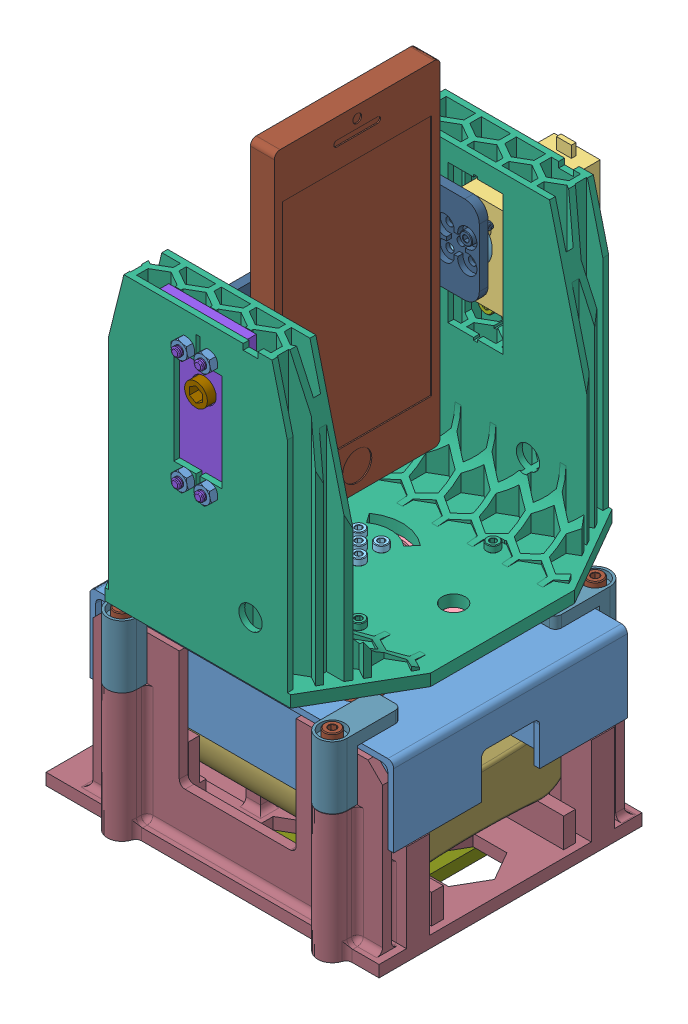
SolidWorks assembly ASSY_IRT_PT_CAM, configuration FIXED. Lengths in mm.
Overall size (144.78 280.29 170.14).
101 component instances, 31 part files, 133 mates.
Components (placement in the parent):
- PAN_BASE_MAIN-1: PAN_BASE_MAIN [Default] at origin
- SPACER_0.75 DIA_8MM-1: SPACER_0.75 DIA_8MM [Default] at (-29.21 34.29 -29.21)
- SPACER_0.75 DIA_8MM-2: SPACER_0.75 DIA_8MM [Default] at (-29.21 34.29 29.21)
- SPACER_0.75 DIA_8MM-3: SPACER_0.75 DIA_8MM [Default] at (29.21 34.29 29.21)
- SPACER_0.75 DIA_8MM-4: SPACER_0.75 DIA_8MM [Default] at (29.21 34.29 -29.21)
- 20KG_6.8V_8V_DIGITAL_SERVO_DSSERVO-1: 20KG_6.8V_8V_DIGITAL_SERVO_DSSERVO [Default] at (-9.464 0.875 0)
- TURNTABLE_ROTATING_ASSY-1: TURNTABLE_ROTATING_ASSY [Default] at (0 42.29 0) size (71.12 8.89 71.12)
  - TURNTABLE_ROTATING_2.8 X 2.8-1: TURNTABLE_ROTATING_2.8 X 2.8 [Default] at origin size (71.12 0.95 71.12)
  - TURNTABLE_ROTATING_2.8 X 2.8-2: TURNTABLE_ROTATING_2.8 X 2.8 [Default] at (0 7.9375 0) x (-1 0 0) z (0 0 -1) size (71.12 0.95 71.12)
- HORN_SERVO-1: HORN_SERVO [Default] at (0 44.3652 0) x (0.996669 0 -0.081556) z (0.081556 0 0.996669)
- TILT_MAIN_BRACKET-1: TILT_MAIN_BRACKET [Default] at (0 51.18 0) x (0 0 1) z (-1 0 0)
- 20KG_6.8V_8V_DIGITAL_SERVO_DSSERVO-2: 20KG_6.8V_8V_DIGITAL_SERVO_DSSERVO [Default] at (0 140.08 -95.01) x (0 1 0) z (1 0 0)
- INNER_COVER_20KG_6.8V_8V_DIGITAL_SERVO_DSSERVO-1: INNER_COVER_20KG_6.8V_8V_DIGITAL_SERVO_DSSERVO [Default] at (0 140.08 60.96)
- COVER_20KG_6.8V_8V_DIGITAL_SERVO_DSSERVO-1: COVER_20KG_6.8V_8V_DIGITAL_SERVO_DSSERVO [Default] at (0 140.08 67.31) x (-1 0 0) z (0 0 -1)
- MOCKUP_LONG_HORN_SERVO-1: MOCKUP_LONG_HORN_SERVO [Default] at (0 149.544 70.705) x (0 1 0) z (-1 0 0)
- HORN_SERVO-2: HORN_SERVO [Default] at (0 149.544 -51.5198) x (0.707107 -0.707107 0) z (-0.707107 -0.707107 0)
- TILT_LONG_BRACKET-1: TILT_LONG_BRACKET [Default] at (-15.24 149.544 -0.415) x (0 0 1) z (0 1 0)
- GALAXY_PHONE-1: GALAXY_PHONE [Default] at (-6.223 149.544 -0.415) x (0 0 -1) z (1 0 0)
- BATTERY_POWER_MASTER_GPCT669-1: BATTERY_POWER_MASTER_GPCT669 [Default] at (0 -13.0494 0) x (0 0 -1) z (1 0 0)
- BASE_BATTERY_ESP32-1: BASE_BATTERY_ESP32 [Default] at (0 -43.8787 0) x (-1 0 0) z (0 0 -1)
- PUSH_DOWN-1: PUSH_DOWN [Default] at (45.72 12.192 52.578) x (-1 0 0) z (0 0 -1)
- PUSH_DOWN-2: PUSH_DOWN [Default] at (-45.72 12.0013 52.578) x (-1 0 0) z (0 0 -1)
- PUSH_DOWN-3: PUSH_DOWN [Default] at (-45.72 12.192 -52.578)
- PUSH_DOWN-4: PUSH_DOWN [Default] at (45.72 12.192 -52.578)
- ESP32-1: ESP32 [Default] at (-50.2285 -31.1787 0)
- TRIPOD_ADAPTER-1: TRIPOD_ADAPTER [Default] at (0 -48.9587 0)
- INSERT_PUSH_DOWN-1: INSERT_PUSH_DOWN [Default] at (45.72 10.5213 -57.15)
- INSERT_PUSH_DOWN-2: INSERT_PUSH_DOWN [Default] at (45.72 10.5213 57.15)
- INSERT_PUSH_DOWN-3: INSERT_PUSH_DOWN [Default] at (-45.72 10.5213 -57.15)
- INSERT_PUSH_DOWN-4: INSERT_PUSH_DOWN [Default] at (-45.72 10.5213 57.15)
- INSERT_CENTER_PUSH_DOWN-1: INSERT_CENTER_PUSH_DOWN [Default] at (0 -33.7187 0)
- M4_Steel Hex Nut_90592A090-1: M4_Steel Hex Nut_90592A090 [90592A090] at (15.286 26.975 5)
- M4_Steel Hex Nut_90592A090-4: M4_Steel Hex Nut_90592A090 [90592A090] at (15.286 26.975 -5)
- M4_Steel Hex Nut_90592A090-3: M4_Steel Hex Nut_90592A090 [90592A090] at (-34.214 26.975 -5)
- M4_Steel Hex Nut_90592A090-2: M4_Steel Hex Nut_90592A090 [90592A090] at (-34.214 26.975 5)
- M3_Steel Hex Nut_90592A085-1: M3_Steel Hex Nut_90592A085 [90592A085] at (-29.21 30.55 -29.21) x (0.956593 0 0.291427) z (-0.291427 0 0.956593)
- M3_General Purpose 18-8 Stainless Steel Washer_98689A112-1: M3_General Purpose 18-8 Stainless Steel Washer_98689A112 [98689A112] at (-29.21 43.5425 -29.21) x (1 0 0) z (0 1 0)
- M3 X 16MM_Button Head Hex Drive Screw_92095A184-1: M3 X 16MM_Button Head Hex Drive Screw_92095A184 [92095A184] at (-29.21 45.4925 -29.21) x (1 0 0) z (0 1 0)
- M3_General Purpose 18-8 Stainless Steel Washer_98689A112-2: M3_General Purpose 18-8 Stainless Steel Washer_98689A112 [98689A112] at (29.21 49.9275 -29.21) x (0.994029 0 -0.109119) z (0 -1 0)
- M3_Steel Hex Nut_90592A085-5: M3_Steel Hex Nut_90592A085 [90592A085] at (29.21 48.4275 -29.21) x (0.873242 0 0.487286) z (-0.487286 0 0.873242)
- M3_Steel Hex Nut_90592A085-9: M3_Steel Hex Nut_90592A085 [90592A085] at (0 149.544 49.6935) x (0.5 0.866025 0) z (-0.866025 0.5 0)
- M3 X 12MM_18-8 Stainless Steel Socket Head Screw_91292A114-1: M3 X 12MM_18-8 Stainless Steel Socket Head Screw_91292A114 [91292A114] at (4.9391 44.26 4.9391) x (1 0 0) z (0 -1 0)
- M3 X 10MM_18-8 Stainless Steel Socket Head Screw_91292A113-1: M3 X 10MM_18-8 Stainless Steel Socket Head Screw_91292A113 [91292A113] at (-29.21 46.26 -29.21) x (-0.837169 0 -0.546944) z (0 -1 0)
- M4 X 10MM_18-8 Stainless Steel Socket Head Screw_91292A116-1: M4 X 10MM_18-8 Stainless Steel Socket Head Screw_91292A116 [91292A116] at (5 164.83 -74.135) x (-1 0 0) z (0 0 -1)
- M4_Steel Hex Nut_90592A090-5: M4_Steel Hex Nut_90592A090 [90592A090] at (5 164.83 -71.45) x (-0.976148 -0.217105 0) z (-0.217105 0.976148 0)
- M4_Steel Hex Nut_90592A090-9: M4_Steel Hex Nut_90592A090 [90592A090] at (5 164.83 71.45) x (-0.976148 -0.217105 0) z (-0.217105 0.976148 0)
- M4 X 14MM_18-8 Stainless Steel Socket Head Screw_91292A038-1: M4 X 14MM_18-8 Stainless Steel Socket Head Screw_91292A038 [91292A038] at (5 164.83 74.96) x (0.908511 -0.417861 0) z (0 0 1)
- M4 X 12MM_Zinc-Plated Alloy Steel Socket Head Screw_90128A214-1: M4 X 12MM_Zinc-Plated Alloy Steel Socket Head Screw_90128A214 [90128A214] at (15.286 22.29 5) x (1 0 0) z (0 -1 0)
- M3 X 8MM_18-8 Stainless Steel Socket Head Screw_91292A112-6: M3 X 8MM_18-8 Stainless Steel Socket Head Screw_91292A112 [91292A112] at (0 149.544 51.795)
- M3 X 8MM_18-8 Stainless Steel Socket Head Screw_91292A112-1: M3 X 8MM_18-8 Stainless Steel Socket Head Screw_91292A112 [91292A112] at (4.9391 154.4831 -52.625) x (-0.943465 -0.331474 0) z (0 0 -1)
- M4 X 12MM_Zinc-Plated Alloy Steel Socket Head Screw_90128A214-4: M4 X 12MM_Zinc-Plated Alloy Steel Socket Head Screw_90128A214 [90128A214] at (15.286 22.29 -5) x (1 0 0) z (0 -1 0)
- M4 X 12MM_Zinc-Plated Alloy Steel Socket Head Screw_90128A214-3: M4 X 12MM_Zinc-Plated Alloy Steel Socket Head Screw_90128A214 [90128A214] at (-34.214 22.29 -5) x (1 0 0) z (0 -1 0)
- M4 X 12MM_Zinc-Plated Alloy Steel Socket Head Screw_90128A214-2: M4 X 12MM_Zinc-Plated Alloy Steel Socket Head Screw_90128A214 [90128A214] at (-34.214 22.29 5) x (1 0 0) z (0 -1 0)
- M4 X 40MM_18-8 Stainless Steel Socket Head Screw_91292A132-1: M4 X 40MM_18-8 Stainless Steel Socket Head Screw_91292A132 [91292A132] at (-45.72 18.37 -57.15) x (1 0 0) z (0 1 0)
- M4 X 40MM_18-8 Stainless Steel Socket Head Screw_91292A132-2: M4 X 40MM_18-8 Stainless Steel Socket Head Screw_91292A132 [91292A132] at (-45.72 18.1793 57.15) x (1 0 0) z (0 1 0)
- M4 X 40MM_18-8 Stainless Steel Socket Head Screw_91292A132-3: M4 X 40MM_18-8 Stainless Steel Socket Head Screw_91292A132 [91292A132] at (45.72 18.37 57.15) x (0.445727 0 0.895169) z (0 1 0)
- M4 X 40MM_18-8 Stainless Steel Socket Head Screw_91292A132-4: M4 X 40MM_18-8 Stainless Steel Socket Head Screw_91292A132 [91292A132] at (45.72 18.37 -57.15) x (0.972297 0 0.23375) z (0 1 0)
- M4_Steel Hex Nut_90592A090-13: M4_Steel Hex Nut_90592A090 [90592A090] at (45.72 8.5213 -57.15) x (0.866025 0 -0.5) z (0.5 0 0.866025)
- M4_Steel Hex Nut_90592A090-14: M4_Steel Hex Nut_90592A090 [90592A090] at (-45.72 8.5213 -57.15) x (0 0 -1) z (1 0 0)
- M4_Steel Hex Nut_90592A090-15: M4_Steel Hex Nut_90592A090 [90592A090] at (45.72 8.5213 57.15) x (0.866025 0 -0.5) z (0.5 0 0.866025)
- M4_Steel Hex Nut_90592A090-16: M4_Steel Hex Nut_90592A090 [90592A090] at (-45.72 8.5213 57.15) x (0.866025 0 -0.5) z (0.5 0 0.866025)
- 1 4 -20_18-8 Stainless Steel Hex Nut_92673A113-1: 1 4 -20_18-8 Stainless Steel Hex Nut_92673A113 [92673A113] at (0 -36.0206 0) x (0.866025 0 0.5) z (0 1 0)
- 1 4 -20 5 AND 8_Zinc-Aluminum-Coated Alloy Steel Socket Head Screw_91274A160-1: 1 4 -20 5 AND 8_Zinc-Aluminum-Coated Alloy Steel Socket Head Screw_91274A160 [91274A160] at (0 -31.3057 0) x (1 0 0) z (0 1 0)
- M3 X 16MM_Button Head Hex Drive Screw_92095A184-2: M3 X 16MM_Button Head Hex Drive Screw_92095A184 [92095A184] at (-29.21 45.4925 29.21) x (1 0 0) z (0 1 0)
- M3 X 16MM_Button Head Hex Drive Screw_92095A184-3: M3 X 16MM_Button Head Hex Drive Screw_92095A184 [92095A184] at (29.21 45.4925 29.21) x (1 0 0) z (0 1 0)
- M3 X 16MM_Button Head Hex Drive Screw_92095A184-4: M3 X 16MM_Button Head Hex Drive Screw_92095A184 [92095A184] at (29.21 45.4925 -29.21) x (1 0 0) z (0 1 0)
- M3_General Purpose 18-8 Stainless Steel Washer_98689A112-3: M3_General Purpose 18-8 Stainless Steel Washer_98689A112 [98689A112] at (29.21 49.9275 29.21) x (0.994029 0 -0.109119) z (0 -1 0)
- M3_General Purpose 18-8 Stainless Steel Washer_98689A112-4: M3_General Purpose 18-8 Stainless Steel Washer_98689A112 [98689A112] at (-29.21 49.9275 29.21) x (0.994029 0 -0.109119) z (0 -1 0)
- M3_General Purpose 18-8 Stainless Steel Washer_98689A112-5: M3_General Purpose 18-8 Stainless Steel Washer_98689A112 [98689A112] at (-29.21 49.9275 -29.21) x (0.994029 0 -0.109119) z (0 -1 0)
- M3_General Purpose 18-8 Stainless Steel Washer_98689A112-6: M3_General Purpose 18-8 Stainless Steel Washer_98689A112 [98689A112] at (-29.21 43.5425 29.21) x (1 0 0) z (0 1 0)
- M3_General Purpose 18-8 Stainless Steel Washer_98689A112-7: M3_General Purpose 18-8 Stainless Steel Washer_98689A112 [98689A112] at (29.21 43.5425 29.21) x (1 0 0) z (0 1 0)
- M3_General Purpose 18-8 Stainless Steel Washer_98689A112-8: M3_General Purpose 18-8 Stainless Steel Washer_98689A112 [98689A112] at (29.21 43.5425 -29.21) x (1 0 0) z (0 1 0)
- M3_Steel Hex Nut_90592A085-2: M3_Steel Hex Nut_90592A085 [90592A085] at (-29.21 30.55 29.21) x (0.956593 0 0.291427) z (-0.291427 0 0.956593)
- M3_Steel Hex Nut_90592A085-3: M3_Steel Hex Nut_90592A085 [90592A085] at (29.21 30.55 29.21) x (0.956593 0 0.291427) z (-0.291427 0 0.956593)
- M3_Steel Hex Nut_90592A085-4: M3_Steel Hex Nut_90592A085 [90592A085] at (29.21 30.55 -29.21) x (0.956593 0 0.291427) z (-0.291427 0 0.956593)
- M3_Steel Hex Nut_90592A085-6: M3_Steel Hex Nut_90592A085 [90592A085] at (29.21 48.4275 29.21) x (0.873242 0 0.487286) z (-0.487286 0 0.873242)
- M3_Steel Hex Nut_90592A085-7: M3_Steel Hex Nut_90592A085 [90592A085] at (-29.21 48.4275 29.21) x (0.873242 0 0.487286) z (-0.487286 0 0.873242)
- M3_Steel Hex Nut_90592A085-8: M3_Steel Hex Nut_90592A085 [90592A085] at (-29.21 48.4275 -29.21) x (0.873242 0 0.487286) z (-0.487286 0 0.873242)
- M3 X 10MM_18-8 Stainless Steel Socket Head Screw_91292A113-2: M3 X 10MM_18-8 Stainless Steel Socket Head Screw_91292A113 [91292A113] at (29.21 46.26 -29.21) x (-0.837169 0 -0.546944) z (0 -1 0)
- M3 X 10MM_18-8 Stainless Steel Socket Head Screw_91292A113-3: M3 X 10MM_18-8 Stainless Steel Socket Head Screw_91292A113 [91292A113] at (29.21 46.26 29.21) x (-0.837169 0 -0.546944) z (0 -1 0)
- M3 X 10MM_18-8 Stainless Steel Socket Head Screw_91292A113-4: M3 X 10MM_18-8 Stainless Steel Socket Head Screw_91292A113 [91292A113] at (-29.21 46.26 29.21) x (-0.837169 0 -0.546944) z (0 -1 0)
- M3 X 12MM_18-8 Stainless Steel Socket Head Screw_91292A114-2: M3 X 12MM_18-8 Stainless Steel Socket Head Screw_91292A114 [91292A114] at (0 44.26 0) x (1 0 0) z (0 -1 0)
- M3 X 12MM_18-8 Stainless Steel Socket Head Screw_91292A114-3: M3 X 12MM_18-8 Stainless Steel Socket Head Screw_91292A114 [91292A114] at (-4.9391 44.26 4.9391) x (1 0 0) z (0 -1 0)
- M3 X 12MM_18-8 Stainless Steel Socket Head Screw_91292A114-4: M3 X 12MM_18-8 Stainless Steel Socket Head Screw_91292A114 [91292A114] at (-4.9391 44.26 -4.9391) x (1 0 0) z (0 -1 0)
- M3 X 12MM_18-8 Stainless Steel Socket Head Screw_91292A114-5: M3 X 12MM_18-8 Stainless Steel Socket Head Screw_91292A114 [91292A114] at (4.9391 44.26 -4.9391) x (1 0 0) z (0 -1 0)
- M4_Steel Hex Nut_90592A090-6: M4_Steel Hex Nut_90592A090 [90592A090] at (5 115.33 -71.45) x (-0.976148 -0.217105 0) z (-0.217105 0.976148 0)
- M4_Steel Hex Nut_90592A090-7: M4_Steel Hex Nut_90592A090 [90592A090] at (-5 115.33 -71.45) x (-0.976148 -0.217105 0) z (-0.217105 0.976148 0)
- M4_Steel Hex Nut_90592A090-8: M4_Steel Hex Nut_90592A090 [90592A090] at (-5 164.83 -71.45) x (-0.976148 -0.217105 0) z (-0.217105 0.976148 0)
- M4 X 10MM_18-8 Stainless Steel Socket Head Screw_91292A116-2: M4 X 10MM_18-8 Stainless Steel Socket Head Screw_91292A116 [91292A116] at (5 115.33 -74.135) x (-1 0 0) z (0 0 -1)
- M4 X 10MM_18-8 Stainless Steel Socket Head Screw_91292A116-3: M4 X 10MM_18-8 Stainless Steel Socket Head Screw_91292A116 [91292A116] at (-5 115.33 -74.135) x (-1 0 0) z (0 0 -1)
- M4 X 10MM_18-8 Stainless Steel Socket Head Screw_91292A116-4: M4 X 10MM_18-8 Stainless Steel Socket Head Screw_91292A116 [91292A116] at (-5 164.83 -74.135) x (-1 0 0) z (0 0 -1)
- M4 X 14MM_18-8 Stainless Steel Socket Head Screw_91292A038-2: M4 X 14MM_18-8 Stainless Steel Socket Head Screw_91292A038 [91292A038] at (-5 115.33 74.96) x (0.908511 -0.417861 0) z (0 0 1)
- M4 X 14MM_18-8 Stainless Steel Socket Head Screw_91292A038-3: M4 X 14MM_18-8 Stainless Steel Socket Head Screw_91292A038 [91292A038] at (5 115.33 74.96) x (0.908511 -0.417861 0) z (0 0 1)
- M4 X 14MM_18-8 Stainless Steel Socket Head Screw_91292A038-4: M4 X 14MM_18-8 Stainless Steel Socket Head Screw_91292A038 [91292A038] at (-5 164.83 74.96) x (0.908511 -0.417861 0) z (0 0 1)
- M4_Steel Hex Nut_90592A090-10: M4_Steel Hex Nut_90592A090 [90592A090] at (-5 115.33 71.45) x (-0.976148 -0.217105 0) z (-0.217105 0.976148 0)
- M4_Steel Hex Nut_90592A090-11: M4_Steel Hex Nut_90592A090 [90592A090] at (5 115.33 71.45) x (-0.976148 -0.217105 0) z (-0.217105 0.976148 0)
- M4_Steel Hex Nut_90592A090-12: M4_Steel Hex Nut_90592A090 [90592A090] at (-5 164.83 71.45) x (-0.976148 -0.217105 0) z (-0.217105 0.976148 0)
- M3 X 8MM_18-8 Stainless Steel Socket Head Screw_91292A112-2: M3 X 8MM_18-8 Stainless Steel Socket Head Screw_91292A112 [91292A112] at (-4.9391 144.6049 -52.625) x (-0.943465 -0.331474 0) z (0 0 -1) (suppressed, hidden)
- M3 X 8MM_18-8 Stainless Steel Socket Head Screw_91292A112-3: M3 X 8MM_18-8 Stainless Steel Socket Head Screw_91292A112 [91292A112] at (-4.9391 154.4831 -52.625) x (-0.943465 -0.331474 0) z (0 0 -1) (suppressed, hidden)
- M3 X 8MM_18-8 Stainless Steel Socket Head Screw_91292A112-4: M3 X 8MM_18-8 Stainless Steel Socket Head Screw_91292A112 [91292A112] at (0 149.544 -52.625) x (-0.943465 -0.331474 0) z (0 0 -1) (suppressed, hidden)
- M3 X 8MM_18-8 Stainless Steel Socket Head Screw_91292A112-5: M3 X 8MM_18-8 Stainless Steel Socket Head Screw_91292A112 [91292A112] at (4.9391 144.6049 -52.625) x (-0.943465 -0.331474 0) z (0 0 -1) (suppressed, hidden)
Mates (geometry in assembly coordinates):
- Coincident1: coincident aligned: plane of BASE_1.3-1 through (0 0 0) normal (1 0 0)
- Coincident2: coincident aligned: plane of BASE_1.3-1 through (0 0 0) normal (0 1 0)
- Coincident3: coincident aligned: plane of BASE_1.3-1 through (0 0 0) normal (0 0 1)
- Concentric1: concentric anti-aligned: cylinder of SPACER_0.75 DIA_8MM-1 through (-29.21 42.29 -29.21) axis (0 -1 0) radius 2; cylinder of BASE_1.3-1 through (-29.21 34.29 -29.21) axis (0 1 0) radius 1.8
- Coincident4: coincident anti-aligned: plane of BASE_1.3-1 through (0 34.29 50.8) normal (0 1 0); plane of SPACER_0.75 DIA_8MM-1 through (-29.21 34.29 -29.21) normal (0 -1 0)
- Parallel1: parallel aligned: plane of SPACER_0.75 DIA_8MM-1 through (-29.21 34.29 -29.21) normal (1 0 0)
- Coincident6: coincident: line of 20KG_6.8V_8V_DIGITAL_SERVO_DSSERVO-1 through (0 46.355 0) axis (0 -1 0)
- Coincident7: coincident anti-aligned: plane of BASE_1.3-1 through (0 31.75 50.8) normal (0 -1 0); plane of 20KG_6.8V_8V_DIGITAL_SERVO_DSSERVO-1 through (-9.464 31.75 0) normal (0 1 0)
- Coincident8: coincident aligned: plane of 20KG_6.8V_8V_DIGITAL_SERVO_DSSERVO-1 through (-9.464 0.875 0) normal (0 0 1)
- Coincident9: coincident anti-aligned: line of BASE_1.3-1 through (15.286 31.75 5) axis (0 1 0); line of M4 X 12MM_Zinc-Plated Alloy Steel Socket Head Screw_90128A214-1 through (15.286 34.29 5) axis (0 -1 0)
- Coincident10: coincident anti-aligned: plane of BASE_1.3-1 through (0 34.29 50.8) normal (0 1 0); plane of M4 X 12MM_Zinc-Plated Alloy Steel Socket Head Screw_90128A214-1 through (15.286 34.29 5) normal (0 -1 0)
- Coincident11: coincident anti-aligned: line of BASE_1.3-1 through (15.286 31.75 5) axis (0 1 0); line of M4 X 3.2MM_Steel Hex Nut_90592A090-1 through (15.286 28.575 5) axis (0 -1 0)
- Coincident12: coincident anti-aligned: plane of 20KG_6.8V_8V_DIGITAL_SERVO_DSSERVO-1 through (-9.464 28.575 0) normal (0 -1 0); plane of M4 X 3.2MM_Steel Hex Nut_90592A090-1 through (11.786 28.575 2.9793) normal (0 1 0)
- Coincident13: coincident anti-aligned: plane of SPACER_0.75 DIA_8MM-3 through (29.21 42.29 29.21) normal (0 1 0); plane of TURNTABLE_ROTATING_ASSY-1/TURNTABLE_ROTATING_2.8 X 2.8-1 through (0 42.29 0) normal (0 -1 0)
- Coincident14: coincident aligned: plane of TURNTABLE_ROTATING_ASSY-1 through (0 42.29 0) normal (1 0 0)
- Coincident15: coincident aligned: plane of TURNTABLE_ROTATING_ASSY-1 through (0 42.29 0) normal (0 0 1)
- Coincident16: coincident anti-aligned: plane of M3 X 16MM_Button Head Hex Drive Screw_92095A184-1 through (-26.36 43.8425 -29.21) normal (0 -1 0); plane of M3_General Purpose 18-8 Stainless Steel Washer_98689A112-1 through (-29.21 43.8425 -29.21) normal (0 1 0)
- Coincident17: coincident anti-aligned: line of BASE_1.3-1 through (-29.21 31.75 -29.21) axis (0 1 0); line of M3_General Purpose 18-8 Stainless Steel Washer_98689A112-1 through (-29.21 43.8425 -29.21) axis (0 -1 0)
- Coincident18: coincident anti-aligned: plane of TURNTABLE_ROTATING_ASSY-1/TURNTABLE_ROTATING_2.8 X 2.8-1 through (0 43.2425 0) normal (0 1 0); plane of M3_General Purpose 18-8 Stainless Steel Washer_98689A112-1 through (-29.21 43.2425 -29.21) normal (0 -1 0)
- Coincident19: coincident anti-aligned: line of BASE_1.3-1 through (-29.21 31.75 -29.21) axis (0 1 0); line of TURNTABLE_ROTATING_ASSY-1/M3_General Purpose 18-8 Stainless Steel Washer_98689A112-1 through (-29.21 43.8425 -29.21) axis (0 -1 0)
- Concentric2: concentric aligned: cylinder of TURNTABLE_ROTATING_ASSY-1/TURNTABLE_ROTATING_2.8 X 2.8-2 through (29.21 51.18 -29.21) axis (0 1 0) radius 1.7; cylinder of M3_General Purpose 18-8 Stainless Steel Washer_98689A112-2 through (29.21 49.6275 -29.21) axis (0 1 0) radius 1.6
- Coincident20: coincident anti-aligned: plane of TURNTABLE_ROTATING_ASSY-1/TURNTABLE_ROTATING_2.8 X 2.8-2 through (0 50.2275 0) normal (0 -1 0); plane of M3_General Purpose 18-8 Stainless Steel Washer_98689A112-2 through (29.21 50.2275 -29.21) normal (0 1 0)
- Coincident21: coincident anti-aligned: line of BASE_1.3-1 through (-29.21 31.75 -29.21) axis (0 1 0); line of M3_Steel Hex Nut_90592A085-1 through (-29.21 31.75 -29.21) axis (0 -1 0)
- Coincident23: coincident anti-aligned: plane of BASE_1.3-1 through (0 31.75 50.8) normal (0 -1 0); plane of M3_Steel Hex Nut_90592A085-1 through (-31.3779 31.75 -31.5302) normal (0 1 0)
- Concentric3: concentric aligned: cylinder of 20KG_6.8V_8V_DIGITAL_SERVO_DSSERVO-1 through (0 46.355 0) axis (0 -1 0) radius 2.921; cylinder of HORN_SERVO-1 through (0 44.3652 0) axis (0 -1 0) radius 4.7244
- Distance2: distance = 18 mm aligned: plane of HORN_SERVO-1 through (0 49.75 0) normal (0 1 0); plane of 20KG_6.8V_8V_DIGITAL_SERVO_DSSERVO-1 through (-9.464 31.75 0) normal (0 1 0)
- Concentric4: concentric aligned: cylinder of TURNTABLE_ROTATING_ASSY-1/TURNTABLE_ROTATING_2.8 X 2.8-2 through (29.21 51.18 29.21) axis (0 1 0) radius 1.7; cylinder of TILT_MAIN_BRACKET-1 through (29.21 56.26 29.21) axis (0 1 0) radius 1.8
- Concentric5: concentric aligned: cylinder of TURNTABLE_ROTATING_ASSY-1/TURNTABLE_ROTATING_2.8 X 2.8-2 through (-29.21 51.18 -29.21) axis (0 1 0) radius 1.7; cylinder of TILT_MAIN_BRACKET-1 through (-29.21 56.26 -29.21) axis (0 1 0) radius 1.8
- Coincident26: coincident anti-aligned: plane of TURNTABLE_ROTATING_ASSY-1/TURNTABLE_ROTATING_2.8 X 2.8-2 through (0 51.18 0) normal (0 1 0); plane of TILT_MAIN_BRACKET-1 through (0 51.18 0) normal (0 -1 0)
- Coincident27: coincident anti-aligned: line of TURNTABLE_ROTATING_ASSY-1/TURNTABLE_ROTATING_2.8 X 2.8-2 through (29.21 50.2275 -29.21) axis (0 1 0); line of M3_Steel Hex Nut_90592A085-5 through (29.21 49.6275 -29.21) axis (0 -1 0)
- Coincident28: coincident anti-aligned: plane of M3_General Purpose 18-8 Stainless Steel Washer_98689A112-2 through (29.21 49.6275 -29.21) normal (0 -1 0); plane of M3_Steel Hex Nut_90592A085-5 through (27.5823 49.6275 -31.9365) normal (0 1 0)
- Coincident33: coincident aligned: line of TILT_MAIN_BRACKET-1 through (-29.21 58.2611 -29.21) axis (0 -1 0); line of M3 X 10MM_18-8 Stainless Steel Socket Head Screw_91292A113-1 through (-29.21 58.985 -29.21) axis (0 -1 0)
- Coincident34: coincident anti-aligned: plane of TILT_MAIN_BRACKET-1 through (0 56.26 0) normal (0 1 0); plane of M3 X 10MM_18-8 Stainless Steel Socket Head Screw_91292A113-1 through (-29.21 56.26 -29.21) normal (0 -1 0)
- Coincident35: coincident anti-aligned: line of TILT_MAIN_BRACKET-1 through (4.9391 51.18 4.9391) axis (0 1 0); line of M3 X 12MM_18-8 Stainless Steel Socket Head Screw_91292A114-1 through (4.9391 58.985 4.9391) axis (0 -1 0)
- Coincident36: coincident anti-aligned: plane of TILT_MAIN_BRACKET-1 through (0 56.26 0) normal (0 1 0); plane of M3 X 12MM_18-8 Stainless Steel Socket Head Screw_91292A114-1 through (4.9391 56.26 4.9391) normal (0 -1 0)
- Coincident37: coincident anti-aligned: plane of TILT_MAIN_BRACKET-1 through (0 51.18 0) normal (-1 0 0); plane of 20KG_6.8V_8V_DIGITAL_SERVO_DSSERVO-2 through (0 140.08 -95.01) normal (1 0 0)
- Concentric6: concentric aligned: cylinder of TILT_MAIN_BRACKET-1 through (-5 164.83 -67.31) axis (0 0 1) radius 2.4; cylinder of 20KG_6.8V_8V_DIGITAL_SERVO_DSSERVO-2 through (-5 164.83 -95.011) axis (0 0 1) radius 2.5
- Concentric7: concentric aligned: cylinder of TILT_MAIN_BRACKET-1 through (5 115.33 -67.31) axis (0 0 1) radius 2.4; cylinder of 20KG_6.8V_8V_DIGITAL_SERVO_DSSERVO-2 through (5 115.33 -95.011) axis (0 0 1) radius 2.5
- Coincident38: coincident anti-aligned: plane of TILT_MAIN_BRACKET-1 through (-101.6 381.3959 -67.31) normal (0 0 1); plane of 20KG_6.8V_8V_DIGITAL_SERVO_DSSERVO-2 through (0 140.08 -67.31) normal (0 0 -1)
- Coincident39: coincident anti-aligned: line of TILT_MAIN_BRACKET-1 through (5 164.83 -69.85) axis (0 0 1); line of M4 X 10MM_18-8 Stainless Steel Socket Head Screw_91292A116-1 through (5 164.83 -60.485) axis (0 0 -1)
- Coincident40: coincident anti-aligned: plane of 20KG_6.8V_8V_DIGITAL_SERVO_DSSERVO-2 through (0 140.08 -64.135) normal (0 0 1); plane of M4 X 10MM_18-8 Stainless Steel Socket Head Screw_91292A116-1 through (5 164.83 -64.135) normal (0 0 -1)
- Coincident41: coincident anti-aligned: line of TILT_MAIN_BRACKET-1 through (5 164.83 -69.85) axis (0 0 1); line of M4_Steel Hex Nut_90592A090-5 through (5 164.83 -69.85) axis (0 0 -1)
- Coincident42: coincident anti-aligned: plane of TILT_MAIN_BRACKET-1 through (-101.6 381.3959 -69.85) normal (0 0 -1); plane of M4_Steel Hex Nut_90592A090-5 through (8.8552 163.6173 -69.85) normal (0 0 1)
- Concentric8: concentric aligned: cylinder of TILT_MAIN_BRACKET-1 through (-5 164.83 67.31) axis (0 0 -1) radius 2.4; cylinder of COVER_20KG_6.8V_8V_DIGITAL_SERVO_DSSERVO-1 through (-5 164.83 63.5) axis (0 0 -1) radius 2.25
- Concentric9: concentric aligned: cylinder of TILT_MAIN_BRACKET-1 through (5 115.33 67.31) axis (0 0 -1) radius 2.4; cylinder of COVER_20KG_6.8V_8V_DIGITAL_SERVO_DSSERVO-1 through (5 115.33 63.5) axis (0 0 -1) radius 2.25
- Coincident43: coincident anti-aligned: plane of TILT_MAIN_BRACKET-1 through (-101.6 381.3959 67.31) normal (0 0 -1); plane of COVER_20KG_6.8V_8V_DIGITAL_SERVO_DSSERVO-1 through (0 140.08 67.31) normal (0 0 1)
- Concentric10: concentric aligned: cylinder of COVER_20KG_6.8V_8V_DIGITAL_SERVO_DSSERVO-1 through (5 164.83 63.5) axis (0 0 -1) radius 2.25; cylinder of INNER_COVER_20KG_6.8V_8V_DIGITAL_SERVO_DSSERVO-1 through (5 164.83 60.96) axis (0 0 -1) radius 2.25
- Concentric11: concentric aligned: cylinder of TILT_MAIN_BRACKET-1 through (5 115.33 67.31) axis (0 0 -1) radius 2.4; cylinder of INNER_COVER_20KG_6.8V_8V_DIGITAL_SERVO_DSSERVO-1 through (5 115.33 60.96) axis (0 0 -1) radius 2.25
- Coincident44: coincident anti-aligned: plane of COVER_20KG_6.8V_8V_DIGITAL_SERVO_DSSERVO-1 through (0 140.08 63.5) normal (0 0 -1); plane of INNER_COVER_20KG_6.8V_8V_DIGITAL_SERVO_DSSERVO-1 through (0 140.08 63.5) normal (0 0 1)
- Coincident47: coincident anti-aligned: line of INNER_COVER_20KG_6.8V_8V_DIGITAL_SERVO_DSSERVO-1 through (5 164.83 63.5) axis (0 0 -1); line of M4 X 14MM_18-8 Stainless Steel Socket Head Screw_91292A038-1 through (5 164.83 60.96) axis (0 0 1)
- Coincident48: coincident anti-aligned: plane of INNER_COVER_20KG_6.8V_8V_DIGITAL_SERVO_DSSERVO-1 through (0 140.08 60.96) normal (0 0 -1); plane of M4 X 14MM_18-8 Stainless Steel Socket Head Screw_91292A038-1 through (5 164.83 60.96) normal (0 0 1)
- Coincident49: coincident aligned: line of INNER_COVER_20KG_6.8V_8V_DIGITAL_SERVO_DSSERVO-1 through (5 164.83 63.5) axis (0 0 -1); line of M4_Steel Hex Nut_90592A090-9 through (5 164.83 73.05) axis (0 0 -1)
- Coincident50: coincident anti-aligned: plane of TILT_MAIN_BRACKET-1 through (-101.6 381.3959 69.85) normal (0 0 1); plane of M4_Steel Hex Nut_90592A090-9 through (8.8552 163.6173 69.85) normal (0 0 -1)
- Concentric12: concentric anti-aligned: cylinder of COVER_20KG_6.8V_8V_DIGITAL_SERVO_DSSERVO-1 through (0 149.544 67.311) axis (0 0 -1) radius 5.3975; cylinder of MOCKUP_LONG_HORN_SERVO-1 through (0 149.544 70.705) axis (0 0 1) radius 4.953
- Concentric13: concentric aligned: cylinder of 20KG_6.8V_8V_DIGITAL_SERVO_DSSERVO-2 through (0 149.544 -49.53) axis (0 0 -1) radius 2.921; cylinder of HORN_SERVO-2 through (0 149.544 -48.5988) axis (0 0 -1) radius 2.667
- Distance3: distance = 18 mm aligned: plane of HORN_SERVO-2 through (0 149.544 -46.135) normal (0 0 1); plane of 20KG_6.8V_8V_DIGITAL_SERVO_DSSERVO-2 through (0 140.08 -64.135) normal (0 0 1)
- Concentric14: concentric aligned: cylinder of HORN_SERVO-2 through (0 149.544 -46.135) axis (0 0 1) radius 1.6; cylinder of TILT_LONG_BRACKET-1 through (0 149.544 -42.325) axis (0 0 1) radius 1.8
- Coincident53: coincident anti-aligned: plane of HORN_SERVO-2 through (0 149.544 -46.135) normal (0 0 1); plane of TILT_LONG_BRACKET-1 through (-11.43 130.494 -46.135) normal (0 0 -1)
- Concentric15: concentric aligned: cylinder of HORN_SERVO-2 through (4.9391 154.4831 -46.135) axis (0 0 1) radius 1.6; cylinder of TILT_LONG_BRACKET-1 through (4.9391 154.4831 -42.325) axis (0 0 1) radius 1.8
- Coincident54: coincident anti-aligned: plane of MOCKUP_LONG_HORN_SERVO-1 through (0 149.544 45.305) normal (0 0 -1); plane of TILT_LONG_BRACKET-1 through (-11.43 130.494 45.305) normal (0 0 1)
- Coincident55: coincident aligned: plane of MOCKUP_LONG_HORN_SERVO-1 through (0 149.544 70.705) normal (0 1 0); plane of TILT_LONG_BRACKET-1 through (-15.24 149.544 -0.415) normal (0 1 0)
- Coincident56: coincident anti-aligned: plane of BASE_BATTERY_ESP32-1 through (0 -43.8787 0) normal (-1 0 0)
- Coincident57: coincident anti-aligned: plane of BASE_BATTERY_ESP32-1 through (0 -43.8787 0) normal (0 0 -1)
- Coincident59: coincident anti-aligned: plane of BASE_BATTERY_ESP32-1 through (0 -43.8787 0) normal (-1 0 0); plane of BATTERY_POWER_MASTER_GPCT669-1 through (0 -13.0494 0) normal (1 0 0)
- Coincident60: coincident aligned: plane of BASE_BATTERY_ESP32-1 through (0 -43.8787 0) normal (0 0 -1); plane of BATTERY_POWER_MASTER_GPCT669-1 through (0 -13.0494 0) normal (0 0 -1)
- Tangent1: tangent anti-aligned: plane of BASE_BATTERY_ESP32-1 through (0 -26.0987 0) normal (0 1 0); cylinder of BATTERY_POWER_MASTER_GPCT669-1 through (52.3875 -13.3987 27.076) axis (1 0 0) radius 12.7
- Tangent2: tangent anti-aligned: plane of BASE_1.3-1 through (66.04 0 50.8) normal (0 -1 0); cylinder of BATTERY_POWER_MASTER_GPCT669-1 through (52.3875 -12.7 27.076) axis (1 0 0) radius 12.7
- Concentric16: concentric aligned: cylinder of PUSH_DOWN-1 through (45.72 39.37 57.15) axis (0 1 0) radius 5.295; cylinder of BASE_BATTERY_ESP32-1 through (45.72 12.0013 57.15) axis (0 1 0) radius 2.4
- Parallel2: parallel anti-aligned: plane of PUSH_DOWN-1 through (45.72 12.192 52.578) normal (-1 0 0)
- Coincident62: coincident anti-aligned: plane of PUSH_DOWN-1 through (45.72 34.29 57.15) normal (0 -1 0); plane of PAN_BASE_MAIN-1 through (0 34.29 50.8) normal (0 1 0)
- Concentric17: concentric aligned: cylinder of BASE_BATTERY_ESP32-1 through (-45.72 12.0013 -57.15) axis (0 1 0) radius 2.4; cylinder of PUSH_DOWN-3 through (-45.72 39.37 -57.15) axis (0 1 0) radius 5.295
- Coincident63: coincident anti-aligned: plane of PAN_BASE_MAIN-1 through (0 34.29 50.8) normal (0 1 0); plane of PUSH_DOWN-3 through (-45.72 34.29 -57.15) normal (0 -1 0)
- Coincident64: coincident anti-aligned: plane of PUSH_DOWN-4 through (45.72 34.29 -57.15) normal (0 -1 0); plane of PAN_BASE_MAIN-1 through (0 34.29 50.8) normal (0 1 0)
- Concentric18: concentric aligned: cylinder of BASE_BATTERY_ESP32-1 through (45.72 12.0013 -57.15) axis (0 1 0) radius 2.4; cylinder of PUSH_DOWN-4 through (45.72 39.37 -57.15) axis (0 1 0) radius 5.295
- Parallel3: parallel aligned: plane of PUSH_DOWN-3 through (-45.72 12.192 -52.578) normal (1 0 0)
- Parallel4: parallel aligned: plane of PUSH_DOWN-4 through (45.72 12.192 -52.578) normal (1 0 0)
- Concentric20: concentric aligned: cylinder of BASE_BATTERY_ESP32-1 through (-45.72 12.0013 57.15) axis (0 1 0) radius 2.4; cylinder of PUSH_DOWN-2 through (-45.72 39.1793 57.15) axis (0 1 0) radius 5.295
- Coincident67: coincident anti-aligned: plane of BASE_BATTERY_ESP32-1 through (-45.72 12.0013 57.15) normal (0 1 0); plane of PUSH_DOWN-2 through (-45.72 12.0013 57.15) normal (0 -1 0)
- Parallel5: parallel anti-aligned: plane of PUSH_DOWN-2 through (-45.72 34.0993 57.15) normal (0 -1 0); plane of PAN_BASE_MAIN-1 through (0 34.29 50.8) normal (0 1 0)
- Parallel6: parallel aligned: plane of ESP32-1 through (-50.2285 -31.1787 0) normal (1 0 0)
- Coincident69: coincident aligned: plane of ESP32-1 through (-50.2285 -31.1787 0) normal (0 0 1)
- Coincident70: coincident anti-aligned: plane of BASE_BATTERY_ESP32-1 through (0 -41.3387 0) normal (0 1 0); plane of ESP32-1 through (-50.2285 -41.3387 0) normal (0 -1 0)
- Coincident71: coincident anti-aligned: plane of BASE_BATTERY_ESP32-1 through (-74.3585 -41.3387 25.4) normal (1 0 0); plane of ESP32-1 through (-74.3585 -29.5277 -13.97) normal (-1 0 0)
- Concentric21: concentric anti-aligned: cylinder of PUSH_DOWN-3 through (-45.72 36.37 -57.15) axis (0 1 0) radius 2.4; cylinder of M4 X 40MM_18-8 Stainless Steel Socket Head Screw_91292A132-1 through (-45.72 -3.63 -57.15) axis (0 -1 0) radius 2
- Coincident72: coincident anti-aligned: plane of PUSH_DOWN-3 through (-43.47 36.37 -57.15) normal (0 1 0); plane of M4 X 40MM_18-8 Stainless Steel Socket Head Screw_91292A132-1 through (-49.045 36.37 -57.15) normal (0 -1 0)
- Concentric22: concentric anti-aligned: cylinder of PUSH_DOWN-4 through (45.72 36.37 -57.15) axis (0 1 0) radius 2.4; cylinder of M4 X 40MM_18-8 Stainless Steel Socket Head Screw_91292A132-4 through (45.72 -3.63 -57.15) axis (0 -1 0) radius 2
- Concentric23: concentric anti-aligned: cylinder of PUSH_DOWN-2 through (-45.72 36.1793 57.15) axis (0 1 0) radius 2.4; cylinder of M4 X 40MM_18-8 Stainless Steel Socket Head Screw_91292A132-2 through (-45.72 -3.8207 57.15) axis (0 -1 0) radius 2
- Concentric24: concentric anti-aligned: cylinder of PUSH_DOWN-1 through (45.72 36.37 57.15) axis (0 1 0) radius 2.4; cylinder of M4 X 40MM_18-8 Stainless Steel Socket Head Screw_91292A132-3 through (45.72 -3.63 57.15) axis (0 -1 0) radius 2
- Coincident73: coincident anti-aligned: plane of PUSH_DOWN-1 through (43.47 36.37 57.15) normal (0 1 0); plane of M4 X 40MM_18-8 Stainless Steel Socket Head Screw_91292A132-3 through (44.238 36.37 54.1736) normal (0 -1 0)
- Coincident74: coincident anti-aligned: plane of PUSH_DOWN-2 through (-47.97 36.1793 57.15) normal (0 1 0); plane of M4 X 40MM_18-8 Stainless Steel Socket Head Screw_91292A132-2 through (-49.045 36.1793 57.15) normal (0 -1 0)
- Coincident75: coincident anti-aligned: plane of PUSH_DOWN-4 through (47.97 36.37 -57.15) normal (0 1 0); plane of M4 X 40MM_18-8 Stainless Steel Socket Head Screw_91292A132-4 through (42.4871 36.37 -57.9272) normal (0 -1 0)
- Parallel7: parallel aligned: plane of TILT_LONG_BRACKET-1 through (-15.24 149.544 -0.415) normal (0 1 0)
- Coincident77: coincident anti-aligned: line of TILT_LONG_BRACKET-1 through (4.9391 154.4831 -44.625) axis (0 0 1); line of M3 X 8MM_18-8 Stainless Steel Socket Head Screw_91292A112-1 through (4.9391 154.4831 -41.9) axis (0 0 -1)
- Coincident78: coincident anti-aligned: plane of TILT_LONG_BRACKET-1 through (-3.1391 144.6049 -44.625) normal (0 0 1); plane of M3 X 8MM_18-8 Stainless Steel Socket Head Screw_91292A112-3 through (-4.9391 154.4831 -44.625) normal (0 0 -1)
- Coincident79: coincident anti-aligned: line of TILT_LONG_BRACKET-1 through (0 149.544 43.795) axis (0 0 -1); line of M3 X 8MM_18-8 Stainless Steel Socket Head Screw_91292A112-6 through (0 149.544 41.07) axis (0 0 1)
- Coincident80: coincident anti-aligned: plane of TILT_LONG_BRACKET-1 through (-3.1391 144.6049 43.795) normal (0 0 -1); plane of M3 X 8MM_18-8 Stainless Steel Socket Head Screw_91292A112-6 through (0 149.544 43.795) normal (0 0 1)
- Coincident81: coincident anti-aligned: line of BASE_BATTERY_ESP32-1 through (45.72 -43.8787 -57.15) axis (0 1 0); line of M4 X 3.2MM_Steel Hex Nut_90592A090-13 through (45.72 10.1213 -57.15) axis (0 -1 0)
- Coincident82: coincident anti-aligned: plane of BASE_BATTERY_ESP32-1 through (0 6.9213 0) normal (0 1 0); plane of M4 X 3.2MM_Steel Hex Nut_90592A090-13 through (41.6785 6.9213 -57.15) normal (0 -1 0)
- Parallel8: parallel anti-aligned: plane of BASE_BATTERY_ESP32-1 through (43.4106 6.9213 -61.15) normal (0.866025 0 0.5); plane of M4 X 3.2MM_Steel Hex Nut_90592A090-13 through (43.6993 10.1213 -60.65) normal (-0.866025 0 -0.5)
- Coincident84: coincident anti-aligned: line of BASE_BATTERY_ESP32-1 through (-45.72 -43.8787 -57.15) axis (0 1 0); line of M4 X 3.2MM_Steel Hex Nut_90592A090-14 through (-45.72 10.1213 -57.15) axis (0 -1 0)
- Parallel9: parallel anti-aligned: plane of BASE_BATTERY_ESP32-1 through (-48.0294 6.9213 -61.15) normal (0.866025 0 0.5); plane of M4 X 3.2MM_Steel Hex Nut_90592A090-14 through (-47.7407 10.1213 -60.65) normal (-0.866025 0 -0.5)
- Coincident86: coincident anti-aligned: plane of BASE_BATTERY_ESP32-1 through (0 6.9213 0) normal (0 1 0); plane of M4 X 3.2MM_Steel Hex Nut_90592A090-14 through (-47.7407 6.9213 -53.65) normal (0 -1 0)
- Coincident87: coincident anti-aligned: line of BASE_BATTERY_ESP32-1 through (45.72 -43.8787 57.15) axis (0 1 0); line of M4 X 3.2MM_Steel Hex Nut_90592A090-15 through (45.72 10.1213 57.15) axis (0 -1 0)
- Parallel10: parallel anti-aligned: plane of BASE_BATTERY_ESP32-1 through (50.3388 6.9213 57.15) normal (-0.866025 0 0.5); plane of M4 X 3.2MM_Steel Hex Nut_90592A090-15 through (49.7615 10.1213 57.15) normal (0.866025 0 -0.5)
- Coincident89: coincident anti-aligned: plane of BASE_BATTERY_ESP32-1 through (0 6.9213 0) normal (0 1 0); plane of M4 X 3.2MM_Steel Hex Nut_90592A090-15 through (41.6785 6.9213 57.15) normal (0 -1 0)
- Coincident90: coincident anti-aligned: line of BASE_BATTERY_ESP32-1 through (-45.72 -43.8787 57.15) axis (0 1 0); line of M4 X 3.2MM_Steel Hex Nut_90592A090-16 through (-45.72 10.1213 57.15) axis (0 -1 0)
- Parallel11: parallel anti-aligned: plane of BASE_BATTERY_ESP32-1 through (-48.0294 6.9213 61.15) normal (0 0 -1); plane of M4 X 3.2MM_Steel Hex Nut_90592A090-16 through (-47.7407 10.1213 60.65) normal (0 0 1)
- Coincident92: coincident anti-aligned: plane of BASE_BATTERY_ESP32-1 through (0 6.9213 0) normal (0 1 0); plane of M4 X 3.2MM_Steel Hex Nut_90592A090-16 through (-49.7615 6.9213 57.15) normal (0 -1 0)
- Coincident93: coincident anti-aligned: line of BASE_BATTERY_ESP32-1 through (0 -43.8787 0) axis (0 1 0); line of 1 4 -20_18-8 Stainless Steel Hex Nut_92673A113-1 through (0 -33.2425 0) axis (0 -1 0)
- Coincident94: coincident anti-aligned: plane of BASE_BATTERY_ESP32-1 through (0 -38.7987 0) normal (0 1 0); plane of 1 4 -20_18-8 Stainless Steel Hex Nut_92673A113-1 through (-3.2079 -38.7987 -5.5563) normal (0 -1 0)
- Parallel12: parallel aligned: plane of BASE_BATTERY_ESP32-1 through (-3.2482 -31.1787 -5.6261) normal (0.866025 0 0.5); plane of 1 4 -20_18-8 Stainless Steel Hex Nut_92673A113-1 through (3.2079 -33.2425 5.5563) normal (0.866025 0 0.5)
- Concentric25: concentric anti-aligned: cylinder of BASE_BATTERY_ESP32-1 through (0 -38.7987 0) axis (0 1 0) radius 3.2639; cylinder of TRIPOD_ADAPTER-1 through (0 -47.1807 0) axis (0 -1 0) radius 3.3782
- Coincident96: coincident anti-aligned: plane of BASE_BATTERY_ESP32-1 through (0 -43.8787 0) normal (0 -1 0); plane of TRIPOD_ADAPTER-1 through (0 -43.8787 0) normal (0 1 0)
- Coincident97: coincident aligned: plane of TRIPOD_ADAPTER-1 through (0 -48.9587 0) normal (0 0 1)
- Concentric27: concentric anti-aligned: cylinder of TRIPOD_ADAPTER-1 through (0 -47.1807 0) axis (0 -1 0) radius 3.3782; cylinder of 1 4 -20 5 AND 8_Zinc-Aluminum-Coated Alloy Steel Socket Head Screw_91274A160-1 through (0 -53.5307 0) axis (0 1 0) radius 4.7625
- Coincident99: coincident anti-aligned: plane of TRIPOD_ADAPTER-1 through (0 -47.1807 0) normal (0 -1 0); plane of 1 4 -20 5 AND 8_Zinc-Aluminum-Coated Alloy Steel Socket Head Screw_91274A160-1 through (0 -47.1807 0) normal (0 1 0)
- Coincident100: coincident anti-aligned: plane of TILT_LONG_BRACKET-1 through (-15.24 149.544 -0.415) normal (0 0 1); plane of GALAXY_PHONE-1 through (-6.223 149.544 -0.415) normal (0 0 -1)
- Coincident101: coincident anti-aligned: plane of TILT_LONG_BRACKET-1 through (-11.43 149.544 -0.415) normal (1 0 0); plane of GALAXY_PHONE-1 through (-11.43 149.544 -0.415) normal (-1 0 0)
- Coincident102: coincident aligned: plane of TILT_LONG_BRACKET-1 through (-15.24 149.544 -0.415) normal (0 1 0); plane of GALAXY_PHONE-1 through (-6.223 149.544 -0.415) normal (0 1 0)
- Coincident103: coincident anti-aligned: plane of TILT_LONG_BRACKET-1 through (-3.1391 144.6049 -44.625) normal (0 0 1); plane of M3 X 8MM_18-8 Stainless Steel Socket Head Screw_91292A112-1 through (4.9391 154.4831 -44.625) normal (0 0 -1)
- Parallel13: parallel anti-aligned: plane of PUSH_DOWN-2 through (-45.72 12.0013 52.578) normal (-1 0 0)
- Coincident104: coincident anti-aligned: plane of BASE_BATTERY_ESP32-1 through (0 10.5213 0) normal (0 1 0); plane of INSERT_PUSH_DOWN-1 through (45.72 10.5213 -57.15) normal (0 -1 0)
- Concentric28: concentric anti-aligned: cylinder of BASE_BATTERY_ESP32-1 through (45.72 31.243 -57.15) axis (0 -1 0) radius 4.7625; cylinder of INSERT_PUSH_DOWN-1 through (45.72 11.4865 -57.15) axis (0 1 0) radius 2.25
- Coincident105: coincident anti-aligned: plane of BASE_BATTERY_ESP32-1 through (0 10.5213 0) normal (0 1 0); plane of INSERT_PUSH_DOWN-3 through (-45.72 10.5213 -57.15) normal (0 -1 0)
- Concentric29: concentric aligned: cylinder of BASE_BATTERY_ESP32-1 through (-45.72 31.243 -57.15) axis (0 -1 0) radius 4.7625; cylinder of INSERT_PUSH_DOWN-3 through (-45.72 11.4865 -57.15) axis (0 -1 0) radius 4.5085
- Coincident107: coincident anti-aligned: plane of BASE_BATTERY_ESP32-1 through (0 10.5213 0) normal (0 1 0); plane of INSERT_PUSH_DOWN-2 through (45.72 10.5213 57.15) normal (0 -1 0)
- Concentric30: concentric aligned: cylinder of BASE_BATTERY_ESP32-1 through (45.72 31.243 57.15) axis (0 -1 0) radius 4.7625; cylinder of INSERT_PUSH_DOWN-2 through (45.72 11.4865 57.15) axis (0 -1 0) radius 4.5085
- Coincident108: coincident anti-aligned: plane of BASE_BATTERY_ESP32-1 through (0 10.5213 0) normal (0 1 0); plane of INSERT_PUSH_DOWN-4 through (-45.72 10.5213 57.15) normal (0 -1 0)
- Concentric31: concentric aligned: cylinder of BASE_BATTERY_ESP32-1 through (-45.72 31.243 57.15) axis (0 -1 0) radius 4.7625; cylinder of INSERT_PUSH_DOWN-4 through (-45.72 11.4865 57.15) axis (0 -1 0) radius 4.5085
- Concentric32: concentric anti-aligned: cylinder of BASE_BATTERY_ESP32-1 through (0 -58.5553 0) axis (0 1 0) radius 6.985; cylinder of INSERT_CENTER_PUSH_DOWN-1 through (0 -31.1787 0) axis (0 -1 0) radius 6.731
- Coincident109: coincident aligned: plane of BASE_BATTERY_ESP32-1 through (0 -31.1787 0) normal (0 1 0); plane of INSERT_CENTER_PUSH_DOWN-1 through (0 -31.1787 0) normal (0 1 0)
- Coincident112: coincident anti-aligned: line of COVER_20KG_6.8V_8V_DIGITAL_SERVO_DSSERVO-1 through (0 149.544 67.31) axis (0 0 -1); line of M3_Steel Hex Nut_90592A085-9 through (0 149.544 48.4935) axis (0 0 1)
- Parallel14: parallel anti-aligned: plane of MOCKUP_LONG_HORN_SERVO-1 through (-2.794 151.1571 38.8012) normal (1 0 0); plane of M3_Steel Hex Nut_90592A085-9 through (-2.75 147.9563 48.4935) normal (-1 0 0)
